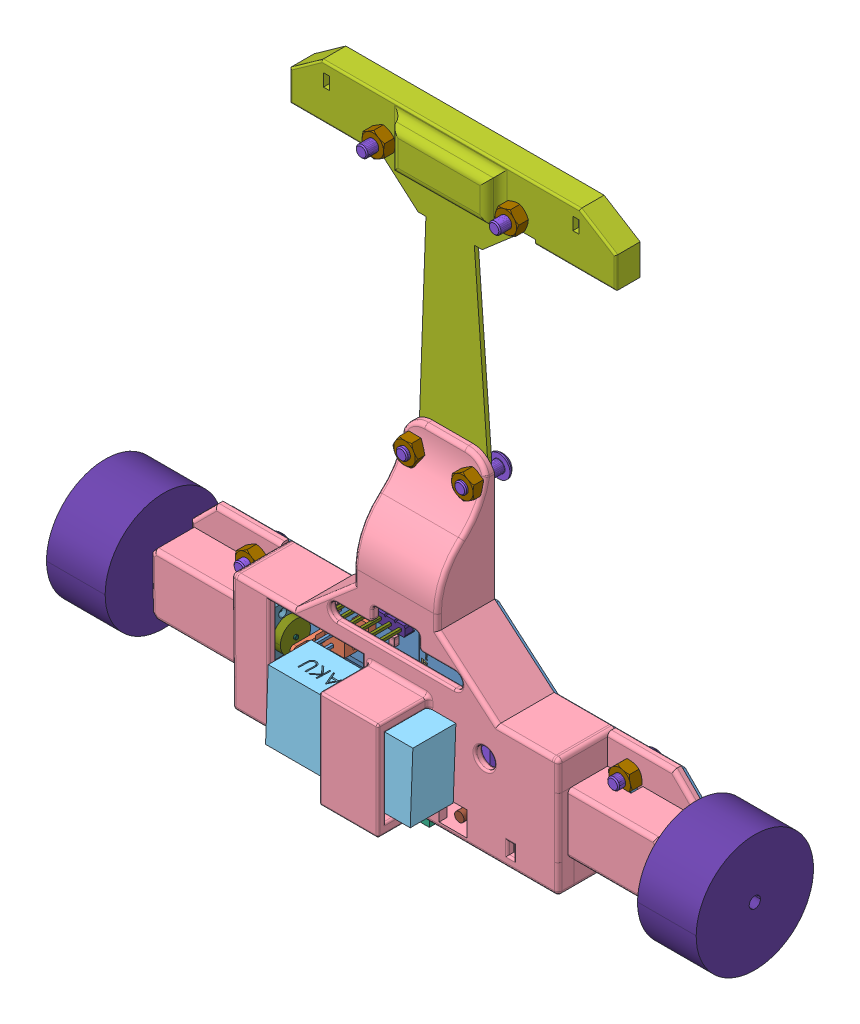
SolidWorks assembly LF_v5_TotalComplexOfRobot, configuration Domyślna. Lengths in mm. (continued)
Components (placement in the parent): (continued)
- LF_v5_MainElectricalBoardwithMCU.step-1: LF_v5_MainElectricalBoardwithMCU.step [Domyślna] at (-21.7771 -53.6224 135.3929) size (166.18 41.84 30.14) (continued)
  - C7FF.step-1: C7FF.step [Domyślna] at origin size (1.35 2.1 1.35)
    - 0805C.step-1: 0805C.step [Domyślna] at (41.8499 9.1411 -1.5914) x (0 -1 0) z (0 0 -1) size (2.1 1.35 1.35)
      - Open CASCADE STEP translator 6.8 2.4.1.1.step-1: Open CASCADE STEP translator 6.8 2.4.1.1.step [Domyślna] at origin size (2.1 1.35 1.35)
      - Open CASCADE STEP translator 6.8 2.4.1.2.step-1: Open CASCADE STEP translator 6.8 2.4.1.2.step [Domyślna] at origin
  - C6FF.step-1: C6FF.step [Domyślna] at origin size (1.35 2.1 1.35)
    - 0805C.step-1: 0805C.step [Domyślna] at (8.1749 19.5091 -1.5914) x (0 -1 0) z (0 0 -1) size (2.1 1.35 1.35)
      - Open CASCADE STEP translator 6.8 2.4.1.1.step-1: Open CASCADE STEP translator 6.8 2.4.1.1.step [Domyślna] at origin size (2.1 1.35 1.35)
      - Open CASCADE STEP translator 6.8 2.4.1.2.step-1: Open CASCADE STEP translator 6.8 2.4.1.2.step [Domyślna] at origin
  - C5FF.step-1: C5FF.step [Domyślna] at origin size (1.35 2.1 1.35)
    - 0805C.step-1: 0805C.step [Domyślna] at (8.1999 14.6341 -1.5914) x (0 -1 0) z (0 0 -1) size (2.1 1.35 1.35)
      - Open CASCADE STEP translator 6.8 2.4.1.1.step-1: Open CASCADE STEP translator 6.8 2.4.1.1.step [Domyślna] at origin size (2.1 1.35 1.35)
      - Open CASCADE STEP translator 6.8 2.4.1.2.step-1: Open CASCADE STEP translator 6.8 2.4.1.2.step [Domyślna] at origin
  - SDDFF.step-1: SDDFF.step [Domyślna] at origin size (14.63 10.38 1)
    - 6479904288.step-1: 6479904288.step [Domyślna] at (3.9409 1.8126 0) size (14.63 10.38 1)
      - Extruded-5.step-1: Extruded-5.step [Domyślna] at origin size (14.63 10.38 1)
  - C3FF.step-1: C3FF.step [Domyślna] at origin size (1.35 2.1 1.35)
    - 0805C.step-1: 0805C.step [Domyślna] at (40.8 7.5091 0) x (0 -1 0) z (0 0 1) size (2.1 1.35 1.35)
      - Open CASCADE STEP translator 6.8 2.4.1.1.step-1: Open CASCADE STEP translator 6.8 2.4.1.1.step [Domyślna] at origin size (2.1 1.35 1.35)
      - Open CASCADE STEP translator 6.8 2.4.1.2.step-1: Open CASCADE STEP translator 6.8 2.4.1.2.step [Domyślna] at origin
  - C2FF.step-1: C2FF.step [Domyślna] at origin size (1.35 2.1 1.35)
    - 0805C.step-1: 0805C.step [Domyślna] at (-4.1751 15.9159 0) x (0 1 0) z (0 0 1) size (2.1 1.35 1.35)
      - Open CASCADE STEP translator 6.8 2.4.1.1.step-1: Open CASCADE STEP translator 6.8 2.4.1.1.step [Domyślna] at origin size (2.1 1.35 1.35)
      - Open CASCADE STEP translator 6.8 2.4.1.2.step-1: Open CASCADE STEP translator 6.8 2.4.1.2.step [Domyślna] at origin
  - J2FF.step-1: J2FF.step [Domyślna] at origin size (15.7 4.25 1.29)
    - 687120183722.step-1: 687120183722.step [Domyślna] at (24.7499 -1.3001 0.64) x (-1 0 0) z (0 0 1) size (15.7 4.25 1.29)
      - 68x120183x22.step-1: 68x120183x22.step [Domyślna] at origin size (13 3.1 1.2)
      - 68X1xx183x22_Pin_Bottom.step-1: 68X1xx183x22_Pin_Bottom.step [Domyślna] at (-4.65 1.05 0.005) x (0 1 0) z (0 0 1) size (3.1 0.2 1.15)
      - 68x120183x22_Actuator.step-1: 68x120183x22_Actuator.step [Domyślna] at (0 -2 0) x (1 0 0) z (0 0 -1) size (15.7 3.8 1.1)
      - 68X1XX183X22_Solder_Pad.step-1: 68X1XX183X22_Solder_Pad.step [Domyślna] at (5.55 -0.25 0.02) x (0 -1 0) z (0 0 1) size (2.5 2 1.24)
      - 68X1xx183x22_Solder_Pad2.step-1: 68X1xx183x22_Solder_Pad2.step [Domyślna] at (-5.55 -0.25 0.02) x (0 -1 0) z (0 0 -1) size (2.5 2 1.24)
      - 68X1xx183x22_Pin_Bottom.step-2: 68X1xx183x22_Pin_Bottom.step [Domyślna] at (-4.15 1.05 0.005) x (0 1 0) z (0 0 1) size (3.1 0.2 1.15)
      - 68X1xx183x22_Pin_Bottom.step-3: 68X1xx183x22_Pin_Bottom.step [Domyślna] at (-3.65 1.05 0.005) x (0 1 0) z (0 0 1) size (3.1 0.2 1.15)
      - 68X1xx183x22_Pin_Bottom.step-4: 68X1xx183x22_Pin_Bottom.step [Domyślna] at (-3.15 1.05 0.005) x (0 1 0) z (0 0 1) size (3.1 0.2 1.15)
      - 68X1xx183x22_Pin_Bottom.step-5: 68X1xx183x22_Pin_Bottom.step [Domyślna] at (-2.65 1.05 0.005) x (0 1 0) z (0 0 1) size (3.1 0.2 1.15)
      - 68X1xx183x22_Pin_Bottom.step-6: 68X1xx183x22_Pin_Bottom.step [Domyślna] at (-2.15 1.05 0.005) x (0 1 0) z (0 0 1) size (3.1 0.2 1.15)
      - 68X1xx183x22_Pin_Bottom.step-7: 68X1xx183x22_Pin_Bottom.step [Domyślna] at (-1.65 1.05 0.005) x (0 1 0) z (0 0 1) size (3.1 0.2 1.15)
      - 68X1xx183x22_Pin_Bottom.step-8: 68X1xx183x22_Pin_Bottom.step [Domyślna] at (-1.15 1.05 0.005) x (0 1 0) z (0 0 1) size (3.1 0.2 1.15)
      - 68X1xx183x22_Pin_Bottom.step-9: 68X1xx183x22_Pin_Bottom.step [Domyślna] at (-0.65 1.05 0.005) x (0 1 0) z (0 0 1) size (3.1 0.2 1.15)
      - 68X1xx183x22_Pin_Bottom.step-10: 68X1xx183x22_Pin_Bottom.step [Domyślna] at (-0.15 1.05 0.005) x (0 1 0) z (0 0 1) size (3.1 0.2 1.15)
      - 68X1xx183x22_Pin_Bottom.step-11: 68X1xx183x22_Pin_Bottom.step [Domyślna] at (0.35 1.05 0.005) x (0 1 0) z (0 0 1) size (3.1 0.2 1.15)
      - 68X1xx183x22_Pin_Bottom.step-12: 68X1xx183x22_Pin_Bottom.step [Domyślna] at (0.85 1.05 0.005) x (0 1 0) z (0 0 1) size (3.1 0.2 1.15)
      - 68X1xx183x22_Pin_Bottom.step-13: 68X1xx183x22_Pin_Bottom.step [Domyślna] at (1.35 1.05 0.005) x (0 1 0) z (0 0 1) size (3.1 0.2 1.15)
      - 68X1xx183x22_Pin_Bottom.step-14: 68X1xx183x22_Pin_Bottom.step [Domyślna] at (1.85 1.05 0.005) x (0 1 0) z (0 0 1) size (3.1 0.2 1.15)
      - 68X1xx183x22_Pin_Bottom.step-15: 68X1xx183x22_Pin_Bottom.step [Domyślna] at (2.35 1.05 0.005) x (0 1 0) z (0 0 1) size (3.1 0.2 1.15)
      - 68X1xx183x22_Pin_Bottom.step-16: 68X1xx183x22_Pin_Bottom.step [Domyślna] at (2.85 1.05 0.005) x (0 1 0) z (0 0 1) size (3.1 0.2 1.15)
      - 68X1xx183x22_Pin_Bottom.step-17: 68X1xx183x22_Pin_Bottom.step [Domyślna] at (3.35 1.05 0.005) x (0 1 0) z (0 0 1) size (3.1 0.2 1.15)
      - 68X1xx183x22_Pin_Bottom.step-18: 68X1xx183x22_Pin_Bottom.step [Domyślna] at (3.85 1.05 0.005) x (0 1 0) z (0 0 1) size (3.1 0.2 1.15)
      - 68X1xx183x22_Pin_Bottom.step-19: 68X1xx183x22_Pin_Bottom.step [Domyślna] at (4.35 1.05 0.005) x (0 1 0) z (0 0 1) size (3.1 0.2 1.15)
      - 68X1xx183x22_Pin_Bottom.step-20: 68X1xx183x22_Pin_Bottom.step [Domyślna] at (4.85 1.05 0.005) x (0 1 0) z (0 0 1) size (3.1 0.2 1.15)
  - J1FF.step-1: J1FF.step [Domyślna] at origin size (15.7 4.25 1.29)
    - 687120183722.step-1: 687120183722.step [Domyślna] at (24.7499 29.4499 0.64) x (-1 0 0) z (0 0 1) size (15.7 4.25 1.29)
      - 68x120183x22.step-1: 68x120183x22.step [Domyślna] at origin size (13 3.1 1.2)
      - 68X1xx183x22_Pin_Bottom.step-1: 68X1xx183x22_Pin_Bottom.step [Domyślna] at (-4.65 1.05 0.005) x (0 1 0) z (0 0 1) size (3.1 0.2 1.15)
      - 68x120183x22_Actuator.step-1: 68x120183x22_Actuator.step [Domyślna] at (0 -2 0) x (1 0 0) z (0 0 -1) size (15.7 3.8 1.1)
      - 68X1XX183X22_Solder_Pad.step-1: 68X1XX183X22_Solder_Pad.step [Domyślna] at (5.55 -0.25 0.02) x (0 -1 0) z (0 0 1) size (2.5 2 1.24)
      - 68X1xx183x22_Solder_Pad2.step-1: 68X1xx183x22_Solder_Pad2.step [Domyślna] at (-5.55 -0.25 0.02) x (0 -1 0) z (0 0 -1) size (2.5 2 1.24)
      - 68X1xx183x22_Pin_Bottom.step-2: 68X1xx183x22_Pin_Bottom.step [Domyślna] at (-4.15 1.05 0.005) x (0 1 0) z (0 0 1) size (3.1 0.2 1.15)
      - 68X1xx183x22_Pin_Bottom.step-3: 68X1xx183x22_Pin_Bottom.step [Domyślna] at (-3.65 1.05 0.005) x (0 1 0) z (0 0 1) size (3.1 0.2 1.15)
      - 68X1xx183x22_Pin_Bottom.step-4: 68X1xx183x22_Pin_Bottom.step [Domyślna] at (-3.15 1.05 0.005) x (0 1 0) z (0 0 1) size (3.1 0.2 1.15)
      - 68X1xx183x22_Pin_Bottom.step-5: 68X1xx183x22_Pin_Bottom.step [Domyślna] at (-2.65 1.05 0.005) x (0 1 0) z (0 0 1) size (3.1 0.2 1.15)
      - 68X1xx183x22_Pin_Bottom.step-6: 68X1xx183x22_Pin_Bottom.step [Domyślna] at (-2.15 1.05 0.005) x (0 1 0) z (0 0 1) size (3.1 0.2 1.15)
      - 68X1xx183x22_Pin_Bottom.step-7: 68X1xx183x22_Pin_Bottom.step [Domyślna] at (-1.65 1.05 0.005) x (0 1 0) z (0 0 1) size (3.1 0.2 1.15)
      - 68X1xx183x22_Pin_Bottom.step-8: 68X1xx183x22_Pin_Bottom.step [Domyślna] at (-1.15 1.05 0.005) x (0 1 0) z (0 0 1) size (3.1 0.2 1.15)
      - 68X1xx183x22_Pin_Bottom.step-9: 68X1xx183x22_Pin_Bottom.step [Domyślna] at (-0.65 1.05 0.005) x (0 1 0) z (0 0 1) size (3.1 0.2 1.15)
      - 68X1xx183x22_Pin_Bottom.step-10: 68X1xx183x22_Pin_Bottom.step [Domyślna] at (-0.15 1.05 0.005) x (0 1 0) z (0 0 1) size (3.1 0.2 1.15)
      - 68X1xx183x22_Pin_Bottom.step-11: 68X1xx183x22_Pin_Bottom.step [Domyślna] at (0.35 1.05 0.005) x (0 1 0) z (0 0 1) size (3.1 0.2 1.15)
      - 68X1xx183x22_Pin_Bottom.step-12: 68X1xx183x22_Pin_Bottom.step [Domyślna] at (0.85 1.05 0.005) x (0 1 0) z (0 0 1) size (3.1 0.2 1.15)
      - 68X1xx183x22_Pin_Bottom.step-13: 68X1xx183x22_Pin_Bottom.step [Domyślna] at (1.35 1.05 0.005) x (0 1 0) z (0 0 1) size (3.1 0.2 1.15)
      - 68X1xx183x22_Pin_Bottom.step-14: 68X1xx183x22_Pin_Bottom.step [Domyślna] at (1.85 1.05 0.005) x (0 1 0) z (0 0 1) size (3.1 0.2 1.15)
      - 68X1xx183x22_Pin_Bottom.step-15: 68X1xx183x22_Pin_Bottom.step [Domyślna] at (2.35 1.05 0.005) x (0 1 0) z (0 0 1) size (3.1 0.2 1.15)
      - 68X1xx183x22_Pin_Bottom.step-16: 68X1xx183x22_Pin_Bottom.step [Domyślna] at (2.85 1.05 0.005) x (0 1 0) z (0 0 1) size (3.1 0.2 1.15)
      - 68X1xx183x22_Pin_Bottom.step-17: 68X1xx183x22_Pin_Bottom.step [Domyślna] at (3.35 1.05 0.005) x (0 1 0) z (0 0 1) size (3.1 0.2 1.15)
      - 68X1xx183x22_Pin_Bottom.step-18: 68X1xx183x22_Pin_Bottom.step [Domyślna] at (3.85 1.05 0.005) x (0 1 0) z (0 0 1) size (3.1 0.2 1.15)
      - 68X1xx183x22_Pin_Bottom.step-19: 68X1xx183x22_Pin_Bottom.step [Domyślna] at (4.35 1.05 0.005) x (0 1 0) z (0 0 1) size (3.1 0.2 1.15)
      - 68X1xx183x22_Pin_Bottom.step-20: 68X1xx183x22_Pin_Bottom.step [Domyślna] at (4.85 1.05 0.005) x (0 1 0) z (0 0 1) size (3.1 0.2 1.15)
  - R26FF.step-1: R26FF.step [Domyślna] at origin size (1.6 3.2 0.6)
    - User_Library-SMD_RESISTOR-11206.step-1: User_Library-SMD_RESISTOR-11206.step [Domyślna] at (14.75 16.451 -1.8962) x (1 0 0) z (0 1 0) size (1.6 0.6 3.2)
  - R25FF.step-1: R25FF.step [Domyślna] at origin size (1.6 3.2 0.6)
    - User_Library-SMD_RESISTOR-11206.step-1: User_Library-SMD_RESISTOR-11206.step [Domyślna] at (-4.6001 4.049 0.3048) x (1 0 0) z (0 -1 0) size (1.6 0.6 3.2)
  - R24FF.step-1: R24FF.step [Domyślna] at origin size (1.6 3.2 0.6)
    - User_Library-SMD_RESISTOR-11206.step-1: User_Library-SMD_RESISTOR-11206.step [Domyślna] at (51.8251 -1.0511 0.3048) x (-1 0 0) z (0 1 0) size (1.6 0.6 3.2)
  - R2FF.step-1: R2FF.step [Domyślna] at origin size (1.6 0.8 0.45)
    - User_Library-SMD_RESISTOR-10603.step-1: User_Library-SMD_RESISTOR-10603.step [Domyślna] at (4.3119 13.6809 0.2159) x (0 -1 0) z (-1 0 0) size (0.8 0.45 1.6)
  - P2FF.step-1: P2FF.step [Domyślna] at origin size (20.32 2.54 11.54)
    - 61300811121.step-1: 61300811121.step [Domyślna] at (5.1499 21.75 1.3) x (-1 0 0) z (0 1 0) size (20.32 11.54 2.54)
      - 6130xx11121_PIN-6.step-1: 6130xx11121_PIN-6.step [Domyślna] at (-8.89 1.5 0) x (1 0 0) z (0 -1 0) size (0.64 0.64 11.54)
      - 6130xx11121_PIN-6.step-2: 6130xx11121_PIN-6.step [Domyślna] at (-6.35 1.5 0) x (1 0 0) z (0 -1 0) size (0.64 0.64 11.54)
      - 6130xx11121_PIN-6.step-3: 6130xx11121_PIN-6.step [Domyślna] at (-3.81 1.5 0) x (1 0 0) z (0 -1 0) size (0.64 0.64 11.54)
      - 6130xx11121_PIN-6.step-4: 6130xx11121_PIN-6.step [Domyślna] at (-1.27 1.5 0) x (1 0 0) z (0 -1 0) size (0.64 0.64 11.54)
      - 6130xx11121_PIN-6.step-5: 6130xx11121_PIN-6.step [Domyślna] at (1.27 1.5 0) x (1 0 0) z (0 -1 0) size (0.64 0.64 11.54)
      - 6130xx11121_PIN-6.step-6: 6130xx11121_PIN-6.step [Domyślna] at (3.81 1.5 0) x (1 0 0) z (0 -1 0) size (0.64 0.64 11.54)
      - 6130xx11121_PIN-6.step-7: 6130xx11121_PIN-6.step [Domyślna] at (6.35 1.5 0) x (1 0 0) z (0 -1 0) size (0.64 0.64 11.54)
      - 6130xx11121_PIN-6.step-8: 6130xx11121_PIN-6.step [Domyślna] at (8.89 1.5 0) x (1 0 0) z (0 -1 0) size (0.64 0.64 11.54)
      - 61300811121-7.step-1: 61300811121-7.step [Domyślna] at origin size (20.32 2.54 2.54)
  - C29FF.step-1: C29FF.step [Domyślna] at origin size (1.71 3.2 1.71)
    - User_Library-Capacitor_Vishay_1206_X7R.step-1: User_Library-Capacitor_Vishay_1206_X7R.step [Domyślna] at (13 25.8148 -0.0102) x (0 1 0) z (0 0 1) size (3.2 1.7 1.7)
  - C22FF.step-1: C22FF.step [Domyślna] at origin size (1.35 2.1 1.35)
    - 0805C.step-1: 0805C.step [Domyślna] at (15.05 26.0802 0) x (0 -1 0) z (0 0 1) size (2.1 1.35 1.35)
      - Open CASCADE STEP translator 6.8 2.4.1.1.step-1: Open CASCADE STEP translator 6.8 2.4.1.1.step [Domyślna] at origin size (2.1 1.35 1.35)
      - Open CASCADE STEP translator 6.8 2.4.1.2.step-1: Open CASCADE STEP translator 6.8 2.4.1.2.step [Domyślna] at origin
  - C21FF.step-1: C21FF.step [Domyślna] at origin size (1.35 2.1 1.35)
    - 0805C.step-1: 0805C.step [Domyślna] at (12.925 10.3641 0) x (0 -1 0) z (0 0 1) size (2.1 1.35 1.35)
      - Open CASCADE STEP translator 6.8 2.4.1.1.step-1: Open CASCADE STEP translator 6.8 2.4.1.1.step [Domyślna] at origin size (2.1 1.35 1.35)
      - Open CASCADE STEP translator 6.8 2.4.1.2.step-1: Open CASCADE STEP translator 6.8 2.4.1.2.step [Domyślna] at origin
  - C20FF.step-1: C20FF.step [Domyślna] at origin size (2.1 1.35 1.35)
    - 0805C.step-1: 0805C.step [Domyślna] at (31.0089 26.0001 0) x (1 0 0) z (0 0 1) size (2.1 1.35 1.35)
      - Open CASCADE STEP translator 6.8 2.4.1.1.step-1: Open CASCADE STEP translator 6.8 2.4.1.1.step [Domyślna] at origin size (2.1 1.35 1.35)
      - Open CASCADE STEP translator 6.8 2.4.1.2.step-1: Open CASCADE STEP translator 6.8 2.4.1.2.step [Domyślna] at origin
  - C14FF.step-1: C14FF.step [Domyślna] at origin size (2.93 3.7 2.03)
    - 3528-SMDB.step-1: 3528-SMDB.step [Domyślna] at (9.2252 0.4759 -1.5914) x (0 -1 0) z (0 0 -1) size (3.7 2.93 2.03)
  - C13FF.step-1: C13FF.step [Domyślna] at origin size (2.93 3.7 2.03)
    - 3528-SMDB.step-1: 3528-SMDB.step [Domyślna] at (-2.7134 0.7259 -1.5914) x (0 -1 0) z (0 0 -1) size (3.7 2.93 2.03)
  - C1FF.step-1: C1FF.step [Domyślna] at origin size (1.35 2.1 1.35)
    - 0805C.step-1: 0805C.step [Domyślna] at (10.6249 15.834 0) x (0 1 0) z (0 0 1) size (2.1 1.35 1.35)
      - Open CASCADE STEP translator 6.8 2.4.1.1.step-1: Open CASCADE STEP translator 6.8 2.4.1.1.step [Domyślna] at origin size (2.1 1.35 1.35)
      - Open CASCADE STEP translator 6.8 2.4.1.2.step-1: Open CASCADE STEP translator 6.8 2.4.1.2.step [Domyślna] at origin
  - U5FF.step-1: U5FF.step [Domyślna] at origin size (16.02 16.02 1.6)
    - IC_STMicroelectronics_STM32H743VIT6_eec.step-1: IC_STMicroelectronics_STM32H743VIT6_eec.step [Domyślna] at (24.75 16.5 0) x (-1 0 0) z (0 0 1) size (16.02 16.02 1.6)
      - Body.step-1: Body.step [Domyślna] at (0 0 0.15) size (14 14 1.45)
      - Leg.step-1: Leg.step [Domyślna] x (1 0 0) z (0 -1 0) size (16.02 0.95 12.22)
      - Leg.step-2: Leg.step [Domyślna] x (0 1 0) z (1 0 0) size (16.02 0.95 12.22)
      - STM_Logo.step-1: STM_Logo.step [Domyślna] at (-2.8487 4.3575 1.501) x (0 1 0) z (0 0 1) size (12.46 12.33 0.1)
- LF_v5_TopHousingPart-1: LF_v5_TopHousingPart [Domyślna] at (-21.7771 -53.6224 135.3929) size (130.04 75.06 27.98)
- LF_v5_BatterySimulationModel-1: LF_v5_BatterySimulationModel [Domyślna] at (161.4668 -18.3015 107.6339) x (0.999287 0.014417 0.034894) z (0 -0.924225 0.381849) size (38.3 18.4 20.84)
- LF_v5_TrackPartSimulation-1: LF_v5_TrackPartSimulation [Domyślna] at (-97.4602 150.0573 127.6146) x (0.000673 -0.99972 -0.023647) z (0 -0.023647 0.99972) size (300 200 3.02) (hidden)
- LF_v5_SwitchOnOffSimulation-1: LF_v5_SwitchOnOffSimulation [Domyślna] at (27.8957 -63.2711 135.3929) x (-1 0 0) z (0 0 1) size (13.5 7 9)
- LF_v5_SensorHousing-2: LF_v5_SensorHousing [Domyślna] at (-21.7771 -53.6224 135.3929) size (83.4 78.08 9.2)
- socket button head cap screw_am-3: socket button head cap screw_am [B18.3.4M - 3 x 0.5 x 10 SBHCS --C] at (-44.8031 -34.8634 130.4514) x (0 0 1) z (-0.850102 -0.526618 0) size (11.65 5.7 5.7)
- socket button head cap screw_am-4: socket button head cap screw_am [B18.3.4M - 3 x 0.5 x 10 SBHCS --C] at (50.7739 -52.8314 130.4514) x (0 0 1) z (-0.953771 -0.300534 0) size (11.65 5.7 5.7)
- socket button head cap screw_am-5: socket button head cap screw_am [B18.3.4M - 3 x 0.5 x 10 SBHCS --C] at (-44.8031 -52.8634 130.4514) x (0 0 1) z (-0.163212 -0.986591 0) size (11.65 5.7 5.7)
- socket button head cap screw_am-6: socket button head cap screw_am [B18.3.4M - 3 x 0.5 x 10 SBHCS --C] at (19.4419 72.0577 129.4514) x (0 0 1) z (-0.390078 -0.920782 0) size (11.65 5.7 5.7)
- socket button head cap screw_am-7: socket button head cap screw_am [B18.3.4M - 3 x 0.5 x 10 SBHCS --C] at (-14.5581 72.0577 129.4514) x (0 0 1) z (0.5735 -0.819206 0) size (11.65 5.7 5.7)
- socket button head cap screw_am-8: socket button head cap screw_am [B18.3.4M - 3 x 0.5 x 10 SBHCS --C] at (10.6625 10.0819 129.4514) x (0 0 1) z (-0.939989 -0.341204 0) size (11.65 5.7 5.7)
- socket button head cap screw_am-9: socket button head cap screw_am [B18.3.4M - 3 x 0.5 x 10 SBHCS --C] at (-4.3375 10.0822 129.4513) x (0 -0.000035 1) z (-0.021567 -0.999767 -0.000035) size (11.65 5.7 5.7)
- socket button head cap screw_am-10: socket button head cap screw_am [B18.3.4M - 3 x 0.5 x 10 SBHCS --C] at (50.7739 -34.8314 130.4514) x (0 0 1) z (0.954106 -0.299469 0) size (11.65 5.7 5.7)
- hex nut style 2_am-1: hex nut style 2_am [B18.2.4.2M - Hex nut, Style 2,  M3 x 0.5 --D-N] at (10.6625 10.0819 140.4256) x (0.999704 0.024347 0) z (0 0 1) size (5.5 6.35 2.9)
- hex nut style 2_am-2: hex nut style 2_am [B18.2.4.2M - Hex nut, Style 2,  M3 x 0.5 --D-N] at (50.7739 -34.8314 137.3929) x (0.967794 0.251745 0) z (0 0 -1) size (5.5 6.35 2.9)
- hex nut style 2_am-3: hex nut style 2_am [B18.2.4.2M - Hex nut, Style 2,  M3 x 0.5 --D-N] at (50.7739 -52.8314 140.2929) size (5.5 6.35 2.9)
- hex nut style 2_am-4: hex nut style 2_am [B18.2.4.2M - Hex nut, Style 2,  M3 x 0.5 --D-N] at (-44.8031 -52.8634 140.2929) size (5.5 6.35 2.9)
- hex nut style 2_am-6: hex nut style 2_am [B18.2.4.2M - Hex nut, Style 2,  M3 x 0.5 --D-N] at (-44.8031 -34.8634 140.2929) size (5.5 6.35 2.9)
- hex nut style 2_am-7: hex nut style 2_am [B18.2.4.2M - Hex nut, Style 2,  M3 x 0.5 --D-N] at (-4.3375 10.0818 140.2251) x (0.866538 -0.49911 -0.000018) z (0 -0.000035 1) size (5.5 6.35 2.9)
- hex nut style 2_am-8: hex nut style 2_am [B18.2.4.2M - Hex nut, Style 2,  M3 x 0.5 --D-N] at (19.4419 72.0577 138.0929) x (0.955349 -0.295479 0) z (0 0 1) size (5.5 6.35 2.9)
- hex nut style 2_am-9: hex nut style 2_am [B18.2.4.2M - Hex nut, Style 2,  M3 x 0.5 --D-N] at (-14.5581 72.0577 138.0929) size (5.5 6.35 2.9)
Mates (geometry in assembly coordinates):
- Wspólnie12: coincident anti-aligned: plane of LF_v5_TopHousingPart-1 through (-21.7771 -53.6224 150.0256) normal (0 0 1); plane of LF_v5_BatterySimulationModel-1 through (161.4668 -18.3015 150.0256) normal (0 0 -1)
- Wspólnie13: coincident anti-aligned: plane of LF_v5_TopHousingPart-1 through (11.6893 -33.4724 161.0256) normal (0 -1 0); plane of LF_v5_BatterySimulationModel-1 through (18.6009 -33.4724 203.2396) normal (0 1 0)
- Koncentryczne4: concentric anti-aligned: circle of LF_v5_ObudowaPlytkiGlownej_CzGorna-1; circle of socket button head cap screw_am-10
- Koncentryczne5: concentric anti-aligned: circle of LF_v5_ObudowaPlytkiGlownej_CzGorna-1; circle of socket button head cap screw_am-4
- Koncentryczne6: concentric anti-aligned: circle of LF_v5_ObudowaPlytkiGlownej_CzGorna-1; circle of socket button head cap screw_am-5
- Koncentryczne7: concentric anti-aligned: circle of LF_v5_ObudowaPlytkiGlownej_CzGorna-1; circle of socket button head cap screw_am-3
- Koncentryczne8: concentric aligned: cylinder of LF_v5_TopHousingPart-1 through (-4.3375 10.0818 141.3938) axis (0 0.000035 -1) radius 1.25; circle of socket button head cap screw_am-9
- Stycznie3: tangent: plane of LF_v5_ObudowaCzescDolna-1 through (-4.3375 10.0819 131.1014) normal (0 0 -1); circle of socket button head cap screw_am-9
- Koncentryczne9: concentric anti-aligned: circle of LF_v5_ObudowaCzescDolna-1; circle of socket button head cap screw_am-8
- Wspólnie30: coincident aligned: plane of LF_v5_ObudowaCzescDolna-1 through (10.6625 10.0819 131.1014) normal (0 0 -1); circle of socket button head cap screw_am-8
- Wspólnie31: coincident anti-aligned: plane of LF_v5_ObudowaCzescDolna-1 through (19.4419 72.0577 131.1014) normal (0 0 -1); plane of socket button head cap screw_am-6 through (18.0608 72.6428 131.1014) normal (0 0 1)
- Wspólnie32: coincident anti-aligned: plane of LF_v5_ObudowaCzescDolna-1 through (-14.5581 72.0577 131.1014) normal (0 0 -1); plane of socket button head cap screw_am-7 through (-15.7869 71.1975 131.1014) normal (0 0 1)
- Wspólnie33: coincident anti-aligned: plane of LF_v5_ObudowaCzescDolna-1 through (-44.8031 -34.8634 132.1014) normal (0 0 -1); plane of socket button head cap screw_am-3 through (-45.593 -33.5883 132.1014) normal (0 0 1)
- Wspólnie34: coincident anti-aligned: plane of LF_v5_ObudowaCzescDolna-1 through (-44.8031 -52.8634 132.1014) normal (0 0 -1); plane of socket button head cap screw_am-5 through (-46.283 -52.6186 132.1014) normal (0 0 1)
- Wspólnie35: coincident anti-aligned: plane of LF_v5_ObudowaCzescDolna-1 through (50.7739 -34.8314 132.1014) normal (0 0 -1); plane of socket button head cap screw_am-10 through (50.3247 -36.2626 132.1014) normal (0 0 1)
- Wspólnie36: coincident anti-aligned: plane of LF_v5_ObudowaCzescDolna-1 through (50.7739 -52.8314 132.1014) normal (0 0 -1); plane of socket button head cap screw_am-4 through (50.3231 -51.4008 132.1014) normal (0 0 1)
- Koncentryczne15: concentric aligned: cylinder of socket button head cap screw_am-10 through (50.7739 -34.8314 130.4514) axis (0 0 -1) radius 1.5; cylinder of hex nut style 2_am-2 through (50.7739 -34.8314 140.2929) axis (0 0 -1) radius 1.25
- Wspólnie38: coincident anti-aligned: plane of LF_v5_TopHousingPart-1 through (-21.7771 -53.6224 137.3929) normal (0 0 1); plane of hex nut style 2_am-2 through (51.5733 -37.9046 137.3929) normal (0 0 -1)
- Koncentryczne16: concentric anti-aligned: cylinder of socket button head cap screw_am-6 through (19.4419 72.0577 129.4514) axis (0 0 -1) radius 1.5; cylinder of hex nut style 2_am-8 through (19.4419 72.0577 135.1929) axis (0 0 1) radius 1.25
- Koncentryczne17: concentric anti-aligned: cylinder of socket button head cap screw_am-7 through (-14.5581 72.0577 129.4514) axis (0 0 -1) radius 1.5; cylinder of hex nut style 2_am-9 through (-14.5581 72.0577 135.1929) axis (0 0 1) radius 1.25
- Koncentryczne18: concentric anti-aligned: cylinder of socket button head cap screw_am-8 through (10.6625 10.0819 129.4514) axis (0 0 -1) radius 1.5; cylinder of hex nut style 2_am-1 through (10.6625 10.0819 137.5256) axis (0 0 1) radius 1.25
- Wspólnie41: coincident anti-aligned: plane of LF_v5_TopHousingPart-1 through (10.6625 10.0819 137.5256) normal (0 0 1); plane of hex nut style 2_am-1 through (10.5852 13.2564 137.5256) normal (0 0 -1)
- Koncentryczne19: concentric anti-aligned: cylinder of socket button head cap screw_am-9 through (-4.3375 10.0822 129.4513) axis (0 0.000035 -1) radius 1.5; cylinder of hex nut style 2_am-7 through (-4.3375 10.0819 137.3251) axis (0 -0.000035 1) radius 1.25
- Stycznie10: tangent: plane of LF_v5_TopHousingPart-1 through (-4.3375 10.0819 137.5256) normal (0 0 1); circle of hex nut style 2_am-7
- Koncentryczne22: concentric anti-aligned: cylinder of socket button head cap screw_am-3 through (-44.8031 -34.8634 130.4514) axis (0 0 -1) radius 1.5; cylinder of hex nut style 2_am-6 through (-44.8031 -34.8634 137.3929) axis (0 0 1) radius 1.25
- Wspólnie44: coincident anti-aligned: plane of LF_v5_TopHousingPart-1 through (-21.7771 -53.6224 137.3929) normal (0 0 1); plane of hex nut style 2_am-6 through (-44.8031 -31.688 137.3929) normal (0 0 -1)
- Koncentryczne23: concentric anti-aligned: cylinder of socket button head cap screw_am-5 through (-44.8031 -52.8634 130.4514) axis (0 0 -1) radius 1.5; cylinder of hex nut style 2_am-4 through (-44.8031 -52.8634 137.3929) axis (0 0 1) radius 1.25
- Wspólnie45: coincident anti-aligned: plane of LF_v5_TopHousingPart-1 through (-21.7771 -53.6224 137.3929) normal (0 0 1); plane of hex nut style 2_am-4 through (-44.8031 -49.688 137.3929) normal (0 0 -1)
- Koncentryczne24: concentric anti-aligned: cylinder of socket button head cap screw_am-4 through (50.7739 -52.8314 130.4514) axis (0 0 -1) radius 1.5; cylinder of hex nut style 2_am-3 through (50.7739 -52.8314 137.3929) axis (0 0 1) radius 1.25
- Wspólnie46: coincident anti-aligned: plane of LF_v5_TopHousingPart-1 through (-21.7771 -53.6224 137.3929) normal (0 0 1); plane of hex nut style 2_am-3 through (50.7739 -49.656 137.3929) normal (0 0 -1)
- Wspólnie53: coincident anti-aligned: plane of LF_v5_TopHousingPart-1 through (-3.6907 -48.9724 139.0256) normal (0 0 1); plane of LF_v5_SwitchOnOffSimulation-1 through (9.8093 -61.9211 139.0256) normal (0 0 -1)
- Wspólnie54: coincident anti-aligned: plane of LF_v5_TopHousingPart-1 through (-3.6907 -48.9724 148.0256) normal (1 0 0); plane of LF_v5_SwitchOnOffSimulation-1 through (-3.6907 -61.9211 139.0256) normal (-1 0 0)
- Wspólnie62: coincident aligned: circle of LF_v5_SensorHousing-2; circle of LF_v5_BoardWithSensors.STEP-1/LFEK_Czujniki_v4P_G.step.STEP-1/BoardCZV.step.STEP-1/Open CASCADE STEP translator 6.8 1.1.1.step.STEP-1
- Wspólnie63: coincident aligned: circle of LF_v5_SensorHousing-2; circle of LF_v5_BoardWithSensors.STEP-1/LFEK_Czujniki_v4P_G.step.STEP-1/BoardCZV.step.STEP-1/Open CASCADE STEP translator 6.8 1.1.1.step.STEP-1
- Wspólnie64: coincident anti-aligned: circle of LF_v5_LowerPartOfHousing-1; circle of LF_v5_BoardWithSensors.STEP-1/LFEK_Czujniki_v4P_G.step.STEP-1/BoardCZV.step.STEP-1/Open CASCADE STEP translator 6.8 1.1.1.step.STEP-1
- Wspólnie65: coincident anti-aligned: circle of LF_v5_LowerPartOfHousing-1; circle of LF_v5_BoardWithSensors.STEP-1/LFEK_Czujniki_v4P_G.step.STEP-1/BoardCZV.step.STEP-1/Open CASCADE STEP translator 6.8 1.1.1.step.STEP-1
